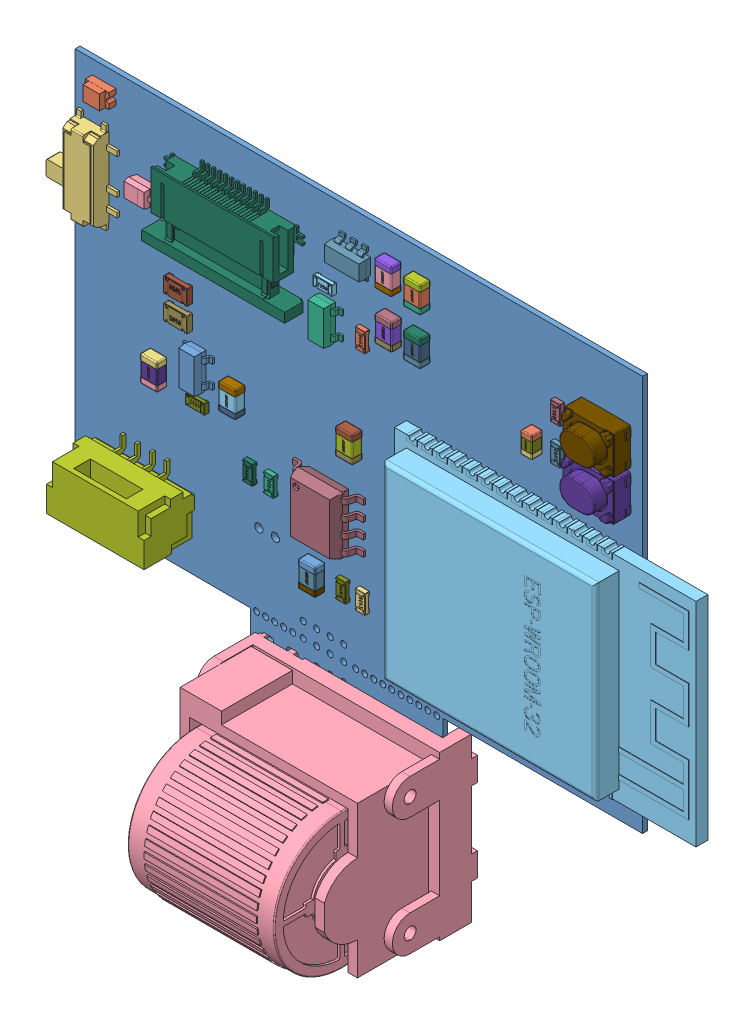
SolidWorks assembly PCB_deskclok_ext_2021-02-23, configuration 默认. Lengths in mm.
Overall size (54.77 48.92 16.75).
124 component instances, 79 part files, 0 mates.
Components (placement in the parent):
- PCB_deskclok_ext_2021-02-23(2)^PCB_deskclok_ext_2021-02-23-1: PCB_deskclok_ext_2021-02-23(2)^PCB_deskclok_ext_2021-02-23 [默认] at origin size (54.77 48.92 16.75) (virtual)
  - Board^PCB_deskclok_ext_2021-02-23(2)_PCB_deskclok_ext_2021-02-23-1: Board^PCB_deskclok_ext_2021-02-23(2)_PCB_deskclok_ext_2021-02-23 [默认] at origin size (48 48.92 0.41) (virtual)
    - Open CASCADE STEP translator 6.8 2.1.1^Board_PCB_deskclok_ext_2021-02-23(2)_PCB_deskclok_ext_2021-02-23-1: Open CASCADE STEP translator 6.8 2.1.1^Board_PCB_deskclok_ext_2021-02-23(2)_PCB_deskclok_ext_2021-02-23 [默认] at (0 0 -0.4115) size (48 48.92 0.41) (virtual)
      - Open CASCADE STEP translator 6.8 2.1.1.1^Open CASCADE STEP translator 6.8 2.1.1_Board_PCB_deskclok_ext_2021-02-23(2)_PCB_deskclok_ext_2021-02-23-1: Open CASCADE STEP translator 6.8 2.1.1.1^Open CASCADE STEP translator 6.8 2.1.1_Board_PCB_deskclok_ext_2021-02-23(2)_PCB_deskclok_ext_2021-02-23 [默认] at origin size (48 48.92 0.41) (virtual)
  - LED6^PCB_deskclok_ext_2021-02-23(2)_PCB_deskclok_ext_2021-02-23-1: LED6^PCB_deskclok_ext_2021-02-23(2)_PCB_deskclok_ext_2021-02-23 [默认] at origin size (2.13 1.25 1.24) (virtual)
    - everlight-17-21-0805LED-GREEN^LED6_PCB_deskclok_ext_2021-02-23(2)_PCB_deskclok_ext_2021-02-23-1: everlight-17-21-0805LED-GREEN^LED6_PCB_deskclok_ext_2021-02-23(2)_PCB_deskclok_ext_2021-02-23 [默认] at (47.3416 90.4196 0.3048) x (1 0 0) z (0 -1 0) size (2.13 1.24 1.25) (virtual)
  - R9^PCB_deskclok_ext_2021-02-23(2)_PCB_deskclok_ext_2021-02-23-1: R9^PCB_deskclok_ext_2021-02-23(2)_PCB_deskclok_ext_2021-02-23 [默认] at origin size (0.8 1.6 0.42) (virtual)
    - User_Library-Res-0603^R9_PCB_deskclok_ext_2021-02-23(2)_PCB_deskclok_ext_2021-02-23-1: User_Library-Res-0603^R9_PCB_deskclok_ext_2021-02-23(2)_PCB_deskclok_ext_2021-02-23 [默认] at (69.3811 64.135 0) x (0 -1 0) z (-1 0 0) size (1.6 0.42 0.8) (virtual)
  - C6^PCB_deskclok_ext_2021-02-23(2)_PCB_deskclok_ext_2021-02-23-1: C6^PCB_deskclok_ext_2021-02-23(2)_PCB_deskclok_ext_2021-02-23 [默认] at origin size (1.45 2.2 0.88) (virtual)
    - c0805c101k5gactu^C6_PCB_deskclok_ext_2021-02-23(2)_PCB_deskclok_ext_2021-02-23-1: c0805c101k5gactu^C6_PCB_deskclok_ext_2021-02-23(2)_PCB_deskclok_ext_2021-02-23 [默认] at (28.223 186.145 -10.6426) x (0 1 0) z (1 0 0) size (2.2 0.88 1.45) (virtual)
      - Open CASCADE STEP translator 6.8 2.4.1.1^c0805c101k5gactu_C6_PCB_deskclok_ext_2021-02-23(2)_PCB_deskclok_ext_2021-02-23-1: Open CASCADE STEP translator 6.8 2.4.1.1^c0805c101k5gactu_C6_PCB_deskclok_ext_2021-02-23(2)_PCB_deskclok_ext_2021-02-23 [默认] at origin size (2 0.86 1.43) (virtual)
      - Open CASCADE STEP translator 6.8 2.4.1.2^c0805c101k5gactu_C6_PCB_deskclok_ext_2021-02-23(2)_PCB_deskclok_ext_2021-02-23-1: Open CASCADE STEP translator 6.8 2.4.1.2^c0805c101k5gactu_C6_PCB_deskclok_ext_2021-02-23(2)_PCB_deskclok_ext_2021-02-23 [默认] at origin size (0.34 0 0.18) (virtual)
      - Open CASCADE STEP translator 6.8 2.4.1.3^c0805c101k5gactu_C6_PCB_deskclok_ext_2021-02-23(2)_PCB_deskclok_ext_2021-02-23-1: Open CASCADE STEP translator 6.8 2.4.1.3^c0805c101k5gactu_C6_PCB_deskclok_ext_2021-02-23(2)_PCB_deskclok_ext_2021-02-23 [默认] at origin size (0.41 0 0.18) (virtual)
      - Open CASCADE STEP translator 6.8 2.4.1.4^c0805c101k5gactu_C6_PCB_deskclok_ext_2021-02-23(2)_PCB_deskclok_ext_2021-02-23-1: Open CASCADE STEP translator 6.8 2.4.1.4^c0805c101k5gactu_C6_PCB_deskclok_ext_2021-02-23(2)_PCB_deskclok_ext_2021-02-23 [默认] at origin size (0.21 0 0.18) (virtual)
      - Open CASCADE STEP translator 6.8 2.4.1.5^c0805c101k5gactu_C6_PCB_deskclok_ext_2021-02-23(2)_PCB_deskclok_ext_2021-02-23-1: Open CASCADE STEP translator 6.8 2.4.1.5^c0805c101k5gactu_C6_PCB_deskclok_ext_2021-02-23(2)_PCB_deskclok_ext_2021-02-23 [默认] at origin size (0.5 0.88 1.45) (virtual)
      - Open CASCADE STEP translator 6.8 2.4.1.6^c0805c101k5gactu_C6_PCB_deskclok_ext_2021-02-23(2)_PCB_deskclok_ext_2021-02-23-1: Open CASCADE STEP translator 6.8 2.4.1.6^c0805c101k5gactu_C6_PCB_deskclok_ext_2021-02-23(2)_PCB_deskclok_ext_2021-02-23 [默认] at origin size (0.5 0.88 1.45) (virtual)
  - C9^PCB_deskclok_ext_2021-02-23(2)_PCB_deskclok_ext_2021-02-23-1: C9^PCB_deskclok_ext_2021-02-23(2)_PCB_deskclok_ext_2021-02-23 [默认] at origin size (1.45 2.2 0.88) (virtual)
    - c0805c101k5gactu^C9_PCB_deskclok_ext_2021-02-23(2)_PCB_deskclok_ext_2021-02-23-1: c0805c101k5gactu^C9_PCB_deskclok_ext_2021-02-23(2)_PCB_deskclok_ext_2021-02-23 [默认] at (117.778 -11.52 -10.6426) x (0 -1 0) z (-1 0 0) size (2.2 0.88 1.45) (virtual)
      - Open CASCADE STEP translator 6.8 2.4.1.1^c0805c101k5gactu_C9_PCB_deskclok_ext_2021-02-23(2)_PCB_deskclok_ext_2021-02-23-1: Open CASCADE STEP translator 6.8 2.4.1.1^c0805c101k5gactu_C9_PCB_deskclok_ext_2021-02-23(2)_PCB_deskclok_ext_2021-02-23 [默认] at origin size (2 0.86 1.43) (virtual)
      - Open CASCADE STEP translator 6.8 2.4.1.2^c0805c101k5gactu_C9_PCB_deskclok_ext_2021-02-23(2)_PCB_deskclok_ext_2021-02-23-1: Open CASCADE STEP translator 6.8 2.4.1.2^c0805c101k5gactu_C9_PCB_deskclok_ext_2021-02-23(2)_PCB_deskclok_ext_2021-02-23 [默认] at origin size (0.34 0 0.18) (virtual)
      - Open CASCADE STEP translator 6.8 2.4.1.3^c0805c101k5gactu_C9_PCB_deskclok_ext_2021-02-23(2)_PCB_deskclok_ext_2021-02-23-1: Open CASCADE STEP translator 6.8 2.4.1.3^c0805c101k5gactu_C9_PCB_deskclok_ext_2021-02-23(2)_PCB_deskclok_ext_2021-02-23 [默认] at origin size (0.41 0 0.18) (virtual)
      - Open CASCADE STEP translator 6.8 2.4.1.4^c0805c101k5gactu_C9_PCB_deskclok_ext_2021-02-23(2)_PCB_deskclok_ext_2021-02-23-1: Open CASCADE STEP translator 6.8 2.4.1.4^c0805c101k5gactu_C9_PCB_deskclok_ext_2021-02-23(2)_PCB_deskclok_ext_2021-02-23 [默认] at origin size (0.21 0 0.18) (virtual)
      - Open CASCADE STEP translator 6.8 2.4.1.5^c0805c101k5gactu_C9_PCB_deskclok_ext_2021-02-23(2)_PCB_deskclok_ext_2021-02-23-1: Open CASCADE STEP translator 6.8 2.4.1.5^c0805c101k5gactu_C9_PCB_deskclok_ext_2021-02-23(2)_PCB_deskclok_ext_2021-02-23 [默认] at origin size (0.5 0.88 1.45) (virtual)
      - Open CASCADE STEP translator 6.8 2.4.1.6^c0805c101k5gactu_C9_PCB_deskclok_ext_2021-02-23(2)_PCB_deskclok_ext_2021-02-23-1: Open CASCADE STEP translator 6.8 2.4.1.6^c0805c101k5gactu_C9_PCB_deskclok_ext_2021-02-23(2)_PCB_deskclok_ext_2021-02-23 [默认] at origin size (0.5 0.88 1.45) (virtual)
  - R1^PCB_deskclok_ext_2021-02-23(2)_PCB_deskclok_ext_2021-02-23-1: R1^PCB_deskclok_ext_2021-02-23(2)_PCB_deskclok_ext_2021-02-23 [默认] at origin size (1.6 0.8 0.42) (virtual)
    - User_Library-Res-0603^R1_PCB_deskclok_ext_2021-02-23(2)_PCB_deskclok_ext_2021-02-23-1: User_Library-Res-0603^R1_PCB_deskclok_ext_2021-02-23(2)_PCB_deskclok_ext_2021-02-23 [默认] at (55.411 71.6281 0) x (1 0 0) z (0 -1 0) size (1.6 0.42 0.8) (virtual)
  - C1^PCB_deskclok_ext_2021-02-23(2)_PCB_deskclok_ext_2021-02-23-1: C1^PCB_deskclok_ext_2021-02-23(2)_PCB_deskclok_ext_2021-02-23 [默认] at origin size (1.45 2.2 0.88) (virtual)
    - c0805c101k5gactu^C1_PCB_deskclok_ext_2021-02-23(2)_PCB_deskclok_ext_2021-02-23-1: c0805c101k5gactu^C1_PCB_deskclok_ext_2021-02-23(2)_PCB_deskclok_ext_2021-02-23 [默认] at (8.411 169.254 -10.6426) x (0 1 0) z (1 0 0) size (2.2 0.88 1.45) (virtual)
      - Open CASCADE STEP translator 6.8 2.4.1.1^c0805c101k5gactu_C1_PCB_deskclok_ext_2021-02-23(2)_PCB_deskclok_ext_2021-02-23-1: Open CASCADE STEP translator 6.8 2.4.1.1^c0805c101k5gactu_C1_PCB_deskclok_ext_2021-02-23(2)_PCB_deskclok_ext_2021-02-23 [默认] at origin size (2 0.86 1.43) (virtual)
      - Open CASCADE STEP translator 6.8 2.4.1.2^c0805c101k5gactu_C1_PCB_deskclok_ext_2021-02-23(2)_PCB_deskclok_ext_2021-02-23-1: Open CASCADE STEP translator 6.8 2.4.1.2^c0805c101k5gactu_C1_PCB_deskclok_ext_2021-02-23(2)_PCB_deskclok_ext_2021-02-23 [默认] at origin size (0.34 0 0.18) (virtual)
      - Open CASCADE STEP translator 6.8 2.4.1.3^c0805c101k5gactu_C1_PCB_deskclok_ext_2021-02-23(2)_PCB_deskclok_ext_2021-02-23-1: Open CASCADE STEP translator 6.8 2.4.1.3^c0805c101k5gactu_C1_PCB_deskclok_ext_2021-02-23(2)_PCB_deskclok_ext_2021-02-23 [默认] at origin size (0.41 0 0.18) (virtual)
      - Open CASCADE STEP translator 6.8 2.4.1.4^c0805c101k5gactu_C1_PCB_deskclok_ext_2021-02-23(2)_PCB_deskclok_ext_2021-02-23-1: Open CASCADE STEP translator 6.8 2.4.1.4^c0805c101k5gactu_C1_PCB_deskclok_ext_2021-02-23(2)_PCB_deskclok_ext_2021-02-23 [默认] at origin size (0.21 0 0.18) (virtual)
      - Open CASCADE STEP translator 6.8 2.4.1.5^c0805c101k5gactu_C1_PCB_deskclok_ext_2021-02-23(2)_PCB_deskclok_ext_2021-02-23-1: Open CASCADE STEP translator 6.8 2.4.1.5^c0805c101k5gactu_C1_PCB_deskclok_ext_2021-02-23(2)_PCB_deskclok_ext_2021-02-23 [默认] at origin size (0.5 0.88 1.45) (virtual)
      - Open CASCADE STEP translator 6.8 2.4.1.6^c0805c101k5gactu_C1_PCB_deskclok_ext_2021-02-23(2)_PCB_deskclok_ext_2021-02-23-1: Open CASCADE STEP translator 6.8 2.4.1.6^c0805c101k5gactu_C1_PCB_deskclok_ext_2021-02-23(2)_PCB_deskclok_ext_2021-02-23 [默认] at origin size (0.5 0.88 1.45) (virtual)
  - C2^PCB_deskclok_ext_2021-02-23(2)_PCB_deskclok_ext_2021-02-23-1: C2^PCB_deskclok_ext_2021-02-23(2)_PCB_deskclok_ext_2021-02-23 [默认] at origin size (1.45 2.2 0.88) (virtual)
    - c0805c101k5gactu^C2_PCB_deskclok_ext_2021-02-23(2)_PCB_deskclok_ext_2021-02-23-1: c0805c101k5gactu^C2_PCB_deskclok_ext_2021-02-23(2)_PCB_deskclok_ext_2021-02-23 [默认] at (15.015 170.524 -10.6426) x (0 1 0) z (1 0 0) size (2.2 0.88 1.45) (virtual)
      - Open CASCADE STEP translator 6.8 2.4.1.1^c0805c101k5gactu_C2_PCB_deskclok_ext_2021-02-23(2)_PCB_deskclok_ext_2021-02-23-1: Open CASCADE STEP translator 6.8 2.4.1.1^c0805c101k5gactu_C2_PCB_deskclok_ext_2021-02-23(2)_PCB_deskclok_ext_2021-02-23 [默认] at origin size (2 0.86 1.43) (virtual)
      - Open CASCADE STEP translator 6.8 2.4.1.2^c0805c101k5gactu_C2_PCB_deskclok_ext_2021-02-23(2)_PCB_deskclok_ext_2021-02-23-1: Open CASCADE STEP translator 6.8 2.4.1.2^c0805c101k5gactu_C2_PCB_deskclok_ext_2021-02-23(2)_PCB_deskclok_ext_2021-02-23 [默认] at origin size (0.34 0 0.18) (virtual)
      - Open CASCADE STEP translator 6.8 2.4.1.3^c0805c101k5gactu_C2_PCB_deskclok_ext_2021-02-23(2)_PCB_deskclok_ext_2021-02-23-1: Open CASCADE STEP translator 6.8 2.4.1.3^c0805c101k5gactu_C2_PCB_deskclok_ext_2021-02-23(2)_PCB_deskclok_ext_2021-02-23 [默认] at origin size (0.41 0 0.18) (virtual)
      - Open CASCADE STEP translator 6.8 2.4.1.4^c0805c101k5gactu_C2_PCB_deskclok_ext_2021-02-23(2)_PCB_deskclok_ext_2021-02-23-1: Open CASCADE STEP translator 6.8 2.4.1.4^c0805c101k5gactu_C2_PCB_deskclok_ext_2021-02-23(2)_PCB_deskclok_ext_2021-02-23 [默认] at origin size (0.21 0 0.18) (virtual)
      - Open CASCADE STEP translator 6.8 2.4.1.5^c0805c101k5gactu_C2_PCB_deskclok_ext_2021-02-23(2)_PCB_deskclok_ext_2021-02-23-1: Open CASCADE STEP translator 6.8 2.4.1.5^c0805c101k5gactu_C2_PCB_deskclok_ext_2021-02-23(2)_PCB_deskclok_ext_2021-02-23 [默认] at origin size (0.5 0.88 1.45) (virtual)
      - Open CASCADE STEP translator 6.8 2.4.1.6^c0805c101k5gactu_C2_PCB_deskclok_ext_2021-02-23(2)_PCB_deskclok_ext_2021-02-23-1: Open CASCADE STEP translator 6.8 2.4.1.6^c0805c101k5gactu_C2_PCB_deskclok_ext_2021-02-23(2)_PCB_deskclok_ext_2021-02-23 [默认] at origin size (0.5 0.88 1.45) (virtual)
  - R13^PCB_deskclok_ext_2021-02-23(2)_PCB_deskclok_ext_2021-02-23-1: R13^PCB_deskclok_ext_2021-02-23(2)_PCB_deskclok_ext_2021-02-23 [默认] at origin size (2 1.25 0.53) (virtual)
    - User_Library-Res-0805^R13_PCB_deskclok_ext_2021-02-23(2)_PCB_deskclok_ext_2021-02-23-1: User_Library-Res-0805^R13_PCB_deskclok_ext_2021-02-23(2)_PCB_deskclok_ext_2021-02-23 [默认] at (54.1409 79.4919 0.3048) x (1 0 0) z (0 -1 0) size (2 0.53 1.25) (virtual)
  - R14^PCB_deskclok_ext_2021-02-23(2)_PCB_deskclok_ext_2021-02-23-1: R14^PCB_deskclok_ext_2021-02-23(2)_PCB_deskclok_ext_2021-02-23 [默认] at origin size (2 1.25 0.53) (virtual)
    - User_Library-Res-0805^R14_PCB_deskclok_ext_2021-02-23(2)_PCB_deskclok_ext_2021-02-23-1: User_Library-Res-0805^R14_PCB_deskclok_ext_2021-02-23(2)_PCB_deskclok_ext_2021-02-23 [默认] at (54.141 77.4801 0.3048) x (-1 0 0) z (0 1 0) size (2 0.53 1.25) (virtual)
  - U3^PCB_deskclok_ext_2021-02-23(2)_PCB_deskclok_ext_2021-02-23-1: U3^PCB_deskclok_ext_2021-02-23(2)_PCB_deskclok_ext_2021-02-23 [默认] at origin size (6 4.9 1.7) (virtual)
    - User_Library-so8-3^U3_PCB_deskclok_ext_2021-02-23(2)_PCB_deskclok_ext_2021-02-23-1: User_Library-so8-3^U3_PCB_deskclok_ext_2021-02-23(2)_PCB_deskclok_ext_2021-02-23 [默认] at (66.4601 69.469 0) x (1 0 0) z (0 0 1) size (6 4.9 1.7) (virtual)
  - U9^PCB_deskclok_ext_2021-02-23(2)_PCB_deskclok_ext_2021-02-23-1: U9^PCB_deskclok_ext_2021-02-23(2)_PCB_deskclok_ext_2021-02-23 [默认] at origin size (3 2.5 1.1) (virtual)
    - CircuitWorks-SOT-23-5^U9_PCB_deskclok_ext_2021-02-23(2)_PCB_deskclok_ext_2021-02-23-1: CircuitWorks-SOT-23-5^U9_PCB_deskclok_ext_2021-02-23(2)_PCB_deskclok_ext_2021-02-23 [默认] at (68.536 88.8961 0.5588) x (-1 0 0) z (0 1 0) size (3 1.1 2.5) (virtual)
  - FPC3^PCB_deskclok_ext_2021-02-23(2)_PCB_deskclok_ext_2021-02-23-1: FPC3^PCB_deskclok_ext_2021-02-23(2)_PCB_deskclok_ext_2021-02-23 [默认] at origin size (12.1 6.6 2) (virtual)
    - 52746-1290_RGB10066329^FPC3_PCB_deskclok_ext_2021-02-23(2)_PCB_deskclok_ext_2021-02-23-1: 52746-1290_RGB10066329^FPC3_PCB_deskclok_ext_2021-02-23(2)_PCB_deskclok_ext_2021-02-23 [默认] at (58.4591 88.7731 0) x (1 0 0) z (0 -1 0) size (12.1 2 6.6) (virtual)
  - C35^PCB_deskclok_ext_2021-02-23(2)_PCB_deskclok_ext_2021-02-23-1: C35^PCB_deskclok_ext_2021-02-23(2)_PCB_deskclok_ext_2021-02-23 [默认] at origin size (0.95 1.77 0.95) (virtual)
    - c0603x104k3ractu^C35_PCB_deskclok_ext_2021-02-23(2)_PCB_deskclok_ext_2021-02-23-1: c0603x104k3ractu^C35_PCB_deskclok_ext_2021-02-23(2)_PCB_deskclok_ext_2021-02-23 [默认] at (40.1705 179.789 -10.6426) x (0 1 0) z (1 0 0) size (1.77 0.95 0.95) (virtual)
      - Open CASCADE STEP translator 6.8 2.14.1.1^c0603x104k3ractu_C35_PCB_deskclok_ext_2021-02-23(2)_PCB_deskclok_ext_2021-02-23-1: Open CASCADE STEP translator 6.8 2.14.1.1^c0603x104k3ractu_C35_PCB_deskclok_ext_2021-02-23(2)_PCB_deskclok_ext_2021-02-23 [默认] at origin size (1.57 0.93 0.93) (virtual)
      - Open CASCADE STEP translator 6.8 2.14.1.2^c0603x104k3ractu_C35_PCB_deskclok_ext_2021-02-23(2)_PCB_deskclok_ext_2021-02-23-1: Open CASCADE STEP translator 6.8 2.14.1.2^c0603x104k3ractu_C35_PCB_deskclok_ext_2021-02-23(2)_PCB_deskclok_ext_2021-02-23 [默认] at origin size (0.24 0 0.13) (virtual)
      - Open CASCADE STEP translator 6.8 2.14.1.3^c0603x104k3ractu_C35_PCB_deskclok_ext_2021-02-23(2)_PCB_deskclok_ext_2021-02-23-1: Open CASCADE STEP translator 6.8 2.14.1.3^c0603x104k3ractu_C35_PCB_deskclok_ext_2021-02-23(2)_PCB_deskclok_ext_2021-02-23 [默认] at origin size (0.29 0 0.13) (virtual)
      - Open CASCADE STEP translator 6.8 2.14.1.4^c0603x104k3ractu_C35_PCB_deskclok_ext_2021-02-23(2)_PCB_deskclok_ext_2021-02-23-1: Open CASCADE STEP translator 6.8 2.14.1.4^c0603x104k3ractu_C35_PCB_deskclok_ext_2021-02-23(2)_PCB_deskclok_ext_2021-02-23 [默认] at origin size (0.15 0 0.13) (virtual)
      - Open CASCADE STEP translator 6.8 2.14.1.5^c0603x104k3ractu_C35_PCB_deskclok_ext_2021-02-23(2)_PCB_deskclok_ext_2021-02-23-1: Open CASCADE STEP translator 6.8 2.14.1.5^c0603x104k3ractu_C35_PCB_deskclok_ext_2021-02-23(2)_PCB_deskclok_ext_2021-02-23 [默认] at origin size (0.45 0.95 0.95) (virtual)
      - Open CASCADE STEP translator 6.8 2.14.1.6^c0603x104k3ractu_C35_PCB_deskclok_ext_2021-02-23(2)_PCB_deskclok_ext_2021-02-23-1: Open CASCADE STEP translator 6.8 2.14.1.6^c0603x104k3ractu_C35_PCB_deskclok_ext_2021-02-23(2)_PCB_deskclok_ext_2021-02-23 [默认] at origin size (0.45 0.95 0.95) (virtual)
  - D1^PCB_deskclok_ext_2021-02-23(2)_PCB_deskclok_ext_2021-02-23-1: D1^PCB_deskclok_ext_2021-02-23(2)_PCB_deskclok_ext_2021-02-23 [默认] at origin size (2.6 1.35 1.1) (virtual)
    - User_Library-SOD323-1^D1_PCB_deskclok_ext_2021-02-23(2)_PCB_deskclok_ext_2021-02-23-1: User_Library-SOD323-1^D1_PCB_deskclok_ext_2021-02-23(2)_PCB_deskclok_ext_2021-02-23 [默认] at (50.9659 85.0899 0) x (-1 0 0) z (0 0 1) size (2.6 1.35 1.1) (virtual)
  - R4^PCB_deskclok_ext_2021-02-23(2)_PCB_deskclok_ext_2021-02-23-1: R4^PCB_deskclok_ext_2021-02-23(2)_PCB_deskclok_ext_2021-02-23 [默认] at origin size (1.6 0.8 0.42) (virtual)
    - User_Library-Res-0603^R4_PCB_deskclok_ext_2021-02-23(2)_PCB_deskclok_ext_2021-02-23-1: User_Library-Res-0603^R4_PCB_deskclok_ext_2021-02-23(2)_PCB_deskclok_ext_2021-02-23 [默认] at (66.2059 85.7249 0) x (-1 0 0) z (0 1 0) size (1.6 0.42 0.8) (virtual)
  - R8^PCB_deskclok_ext_2021-02-23(2)_PCB_deskclok_ext_2021-02-23-1: R8^PCB_deskclok_ext_2021-02-23(2)_PCB_deskclok_ext_2021-02-23 [默认] at origin size (0.8 1.6 0.42) (virtual)
    - User_Library-Res-0603^R8_PCB_deskclok_ext_2021-02-23(2)_PCB_deskclok_ext_2021-02-23-1: User_Library-Res-0603^R8_PCB_deskclok_ext_2021-02-23(2)_PCB_deskclok_ext_2021-02-23 [默认] at (61.6341 68.834 0) x (0 -1 0) z (-1 0 0) size (1.6 0.42 0.8) (virtual)
  - C4^PCB_deskclok_ext_2021-02-23(2)_PCB_deskclok_ext_2021-02-23-1: C4^PCB_deskclok_ext_2021-02-23(2)_PCB_deskclok_ext_2021-02-23 [默认] at origin size (1.45 2.2 0.88) (virtual)
    - c0805c101k5gactu^C4_PCB_deskclok_ext_2021-02-23(2)_PCB_deskclok_ext_2021-02-23-1: c0805c101k5gactu^C4_PCB_deskclok_ext_2021-02-23(2)_PCB_deskclok_ext_2021-02-23 [默认] at (24.921 172.175 -10.6426) x (0 1 0) z (1 0 0) size (2.2 0.88 1.45) (virtual)
      - Open CASCADE STEP translator 6.8 2.4.1.1^c0805c101k5gactu_C4_PCB_deskclok_ext_2021-02-23(2)_PCB_deskclok_ext_2021-02-23-1: Open CASCADE STEP translator 6.8 2.4.1.1^c0805c101k5gactu_C4_PCB_deskclok_ext_2021-02-23(2)_PCB_deskclok_ext_2021-02-23 [默认] at origin size (2 0.86 1.43) (virtual)
      - Open CASCADE STEP translator 6.8 2.4.1.2^c0805c101k5gactu_C4_PCB_deskclok_ext_2021-02-23(2)_PCB_deskclok_ext_2021-02-23-1: Open CASCADE STEP translator 6.8 2.4.1.2^c0805c101k5gactu_C4_PCB_deskclok_ext_2021-02-23(2)_PCB_deskclok_ext_2021-02-23 [默认] at origin size (0.34 0 0.18) (virtual)
      - Open CASCADE STEP translator 6.8 2.4.1.3^c0805c101k5gactu_C4_PCB_deskclok_ext_2021-02-23(2)_PCB_deskclok_ext_2021-02-23-1: Open CASCADE STEP translator 6.8 2.4.1.3^c0805c101k5gactu_C4_PCB_deskclok_ext_2021-02-23(2)_PCB_deskclok_ext_2021-02-23 [默认] at origin size (0.41 0 0.18) (virtual)
      - Open CASCADE STEP translator 6.8 2.4.1.4^c0805c101k5gactu_C4_PCB_deskclok_ext_2021-02-23(2)_PCB_deskclok_ext_2021-02-23-1: Open CASCADE STEP translator 6.8 2.4.1.4^c0805c101k5gactu_C4_PCB_deskclok_ext_2021-02-23(2)_PCB_deskclok_ext_2021-02-23 [默认] at origin size (0.21 0 0.18) (virtual)
      - Open CASCADE STEP translator 6.8 2.4.1.5^c0805c101k5gactu_C4_PCB_deskclok_ext_2021-02-23(2)_PCB_deskclok_ext_2021-02-23-1: Open CASCADE STEP translator 6.8 2.4.1.5^c0805c101k5gactu_C4_PCB_deskclok_ext_2021-02-23(2)_PCB_deskclok_ext_2021-02-23 [默认] at origin size (0.5 0.88 1.45) (virtual)
      - Open CASCADE STEP translator 6.8 2.4.1.6^c0805c101k5gactu_C4_PCB_deskclok_ext_2021-02-23(2)_PCB_deskclok_ext_2021-02-23-1: Open CASCADE STEP translator 6.8 2.4.1.6^c0805c101k5gactu_C4_PCB_deskclok_ext_2021-02-23(2)_PCB_deskclok_ext_2021-02-23 [默认] at origin size (0.5 0.88 1.45) (virtual)
  - R7^PCB_deskclok_ext_2021-02-23(2)_PCB_deskclok_ext_2021-02-23-1: R7^PCB_deskclok_ext_2021-02-23(2)_PCB_deskclok_ext_2021-02-23 [默认] at origin size (0.8 1.6 0.42) (virtual)
    - User_Library-Res-0603^R7_PCB_deskclok_ext_2021-02-23(2)_PCB_deskclok_ext_2021-02-23-1: User_Library-Res-0603^R7_PCB_deskclok_ext_2021-02-23(2)_PCB_deskclok_ext_2021-02-23 [默认] at (85.8909 86.233 0) x (0 1 0) z (1 0 0) size (1.6 0.42 0.8) (virtual)
  - R6^PCB_deskclok_ext_2021-02-23(2)_PCB_deskclok_ext_2021-02-23-1: R6^PCB_deskclok_ext_2021-02-23(2)_PCB_deskclok_ext_2021-02-23 [默认] at origin size (0.8 1.6 0.42) (virtual)
    - User_Library-Res-0603^R6_PCB_deskclok_ext_2021-02-23(2)_PCB_deskclok_ext_2021-02-23-1: User_Library-Res-0603^R6_PCB_deskclok_ext_2021-02-23(2)_PCB_deskclok_ext_2021-02-23 [默认] at (85.8911 83.185 0) x (0 -1 0) z (-1 0 0) size (1.6 0.42 0.8) (virtual)
  - R3^PCB_deskclok_ext_2021-02-23(2)_PCB_deskclok_ext_2021-02-23-1: R3^PCB_deskclok_ext_2021-02-23(2)_PCB_deskclok_ext_2021-02-23 [默认] at origin size (0.8 1.6 0.42) (virtual)
    - User_Library-Res-0603^R3_PCB_deskclok_ext_2021-02-23(2)_PCB_deskclok_ext_2021-02-23-1: User_Library-Res-0603^R3_PCB_deskclok_ext_2021-02-23(2)_PCB_deskclok_ext_2021-02-23 [默认] at (59.8559 68.834 0) x (0 1 0) z (1 0 0) size (1.6 0.42 0.8) (virtual)
  - R2^PCB_deskclok_ext_2021-02-23(2)_PCB_deskclok_ext_2021-02-23-1: R2^PCB_deskclok_ext_2021-02-23(2)_PCB_deskclok_ext_2021-02-23 [默认] at origin size (0.8 1.6 0.42) (virtual)
    - User_Library-Res-0603^R2_PCB_deskclok_ext_2021-02-23(2)_PCB_deskclok_ext_2021-02-23-1: User_Library-Res-0603^R2_PCB_deskclok_ext_2021-02-23(2)_PCB_deskclok_ext_2021-02-23 [默认] at (67.7301 64.135 0) x (0 -1 0) z (-1 0 0) size (1.6 0.42 0.8) (virtual)
  - SW1^PCB_deskclok_ext_2021-02-23(2)_PCB_deskclok_ext_2021-02-23-1: SW1^PCB_deskclok_ext_2021-02-23(2)_PCB_deskclok_ext_2021-02-23 [默认] at origin size (4.6 3.2 2.5) (virtual)
    - skrpace010_RGB10066329^SW1_PCB_deskclok_ext_2021-02-23(2)_PCB_deskclok_ext_2021-02-23-1: skrpace010_RGB10066329^SW1_PCB_deskclok_ext_2021-02-23(2)_PCB_deskclok_ext_2021-02-23 [默认] at (89.8279 83.185 0) x (-1 0 0) z (0 1 0) size (4.6 2.5 3.2) (virtual)
  - SW2^PCB_deskclok_ext_2021-02-23(2)_PCB_deskclok_ext_2021-02-23-1: SW2^PCB_deskclok_ext_2021-02-23(2)_PCB_deskclok_ext_2021-02-23 [默认] at origin size (4.6 3.2 2.5) (virtual)
    - skrpace010_RGB10066329^SW2_PCB_deskclok_ext_2021-02-23(2)_PCB_deskclok_ext_2021-02-23-1: skrpace010_RGB10066329^SW2_PCB_deskclok_ext_2021-02-23(2)_PCB_deskclok_ext_2021-02-23 [默认] at (89.8281 86.614 0) x (1 0 0) z (0 -1 0) size (4.6 2.5 3.2) (virtual)
  - U1^PCB_deskclok_ext_2021-02-23(2)_PCB_deskclok_ext_2021-02-23-1: U1^PCB_deskclok_ext_2021-02-23(2)_PCB_deskclok_ext_2021-02-23 [默认] at origin size (2.5 3 1.1) (virtual)
    - CircuitWorks-SOT-23-5^U1_PCB_deskclok_ext_2021-02-23(2)_PCB_deskclok_ext_2021-02-23-1: CircuitWorks-SOT-23-5^U1_PCB_deskclok_ext_2021-02-23(2)_PCB_deskclok_ext_2021-02-23 [默认] at (55.4148 74.339 0.5588) x (0 -1 0) z (-1 0 0) size (3 1.1 2.5) (virtual)
  - C7^PCB_deskclok_ext_2021-02-23(2)_PCB_deskclok_ext_2021-02-23-1: C7^PCB_deskclok_ext_2021-02-23(2)_PCB_deskclok_ext_2021-02-23 [默认] at origin size (1.45 2.2 0.88) (virtual)
    - c0805c101k5gactu^C7_PCB_deskclok_ext_2021-02-23(2)_PCB_deskclok_ext_2021-02-23-1: c0805c101k5gactu^C7_PCB_deskclok_ext_2021-02-23(2)_PCB_deskclok_ext_2021-02-23 [默认] at (117.778 -7.583 -10.6426) x (0 -1 0) z (-1 0 0) size (2.2 0.88 1.45) (virtual)
      - Open CASCADE STEP translator 6.8 2.4.1.1^c0805c101k5gactu_C7_PCB_deskclok_ext_2021-02-23(2)_PCB_deskclok_ext_2021-02-23-1: Open CASCADE STEP translator 6.8 2.4.1.1^c0805c101k5gactu_C7_PCB_deskclok_ext_2021-02-23(2)_PCB_deskclok_ext_2021-02-23 [默认] at origin size (2 0.86 1.43) (virtual)
      - Open CASCADE STEP translator 6.8 2.4.1.2^c0805c101k5gactu_C7_PCB_deskclok_ext_2021-02-23(2)_PCB_deskclok_ext_2021-02-23-1: Open CASCADE STEP translator 6.8 2.4.1.2^c0805c101k5gactu_C7_PCB_deskclok_ext_2021-02-23(2)_PCB_deskclok_ext_2021-02-23 [默认] at origin size (0.34 0 0.18) (virtual)
      - Open CASCADE STEP translator 6.8 2.4.1.3^c0805c101k5gactu_C7_PCB_deskclok_ext_2021-02-23(2)_PCB_deskclok_ext_2021-02-23-1: Open CASCADE STEP translator 6.8 2.4.1.3^c0805c101k5gactu_C7_PCB_deskclok_ext_2021-02-23(2)_PCB_deskclok_ext_2021-02-23 [默认] at origin size (0.41 0 0.18) (virtual)
      - Open CASCADE STEP translator 6.8 2.4.1.4^c0805c101k5gactu_C7_PCB_deskclok_ext_2021-02-23(2)_PCB_deskclok_ext_2021-02-23-1: Open CASCADE STEP translator 6.8 2.4.1.4^c0805c101k5gactu_C7_PCB_deskclok_ext_2021-02-23(2)_PCB_deskclok_ext_2021-02-23 [默认] at origin size (0.21 0 0.18) (virtual)
      - Open CASCADE STEP translator 6.8 2.4.1.5^c0805c101k5gactu_C7_PCB_deskclok_ext_2021-02-23(2)_PCB_deskclok_ext_2021-02-23-1: Open CASCADE STEP translator 6.8 2.4.1.5^c0805c101k5gactu_C7_PCB_deskclok_ext_2021-02-23(2)_PCB_deskclok_ext_2021-02-23 [默认] at origin size (0.5 0.88 1.45) (virtual)
      - Open CASCADE STEP translator 6.8 2.4.1.6^c0805c101k5gactu_C7_PCB_deskclok_ext_2021-02-23(2)_PCB_deskclok_ext_2021-02-23-1: Open CASCADE STEP translator 6.8 2.4.1.6^c0805c101k5gactu_C7_PCB_deskclok_ext_2021-02-23(2)_PCB_deskclok_ext_2021-02-23 [默认] at origin size (0.5 0.88 1.45) (virtual)
  - C8^PCB_deskclok_ext_2021-02-23(2)_PCB_deskclok_ext_2021-02-23-1: C8^PCB_deskclok_ext_2021-02-23(2)_PCB_deskclok_ext_2021-02-23 [默认] at origin size (1.45 2.2 0.88) (virtual)
    - c0805c101k5gactu^C8_PCB_deskclok_ext_2021-02-23(2)_PCB_deskclok_ext_2021-02-23-1: c0805c101k5gactu^C8_PCB_deskclok_ext_2021-02-23(2)_PCB_deskclok_ext_2021-02-23 [默认] at (115.365 -11.52 -10.6426) x (0 -1 0) z (-1 0 0) size (2.2 0.88 1.45) (virtual)
      - Open CASCADE STEP translator 6.8 2.4.1.1^c0805c101k5gactu_C8_PCB_deskclok_ext_2021-02-23(2)_PCB_deskclok_ext_2021-02-23-1: Open CASCADE STEP translator 6.8 2.4.1.1^c0805c101k5gactu_C8_PCB_deskclok_ext_2021-02-23(2)_PCB_deskclok_ext_2021-02-23 [默认] at origin size (2 0.86 1.43) (virtual)
      - Open CASCADE STEP translator 6.8 2.4.1.2^c0805c101k5gactu_C8_PCB_deskclok_ext_2021-02-23(2)_PCB_deskclok_ext_2021-02-23-1: Open CASCADE STEP translator 6.8 2.4.1.2^c0805c101k5gactu_C8_PCB_deskclok_ext_2021-02-23(2)_PCB_deskclok_ext_2021-02-23 [默认] at origin size (0.34 0 0.18) (virtual)
      - Open CASCADE STEP translator 6.8 2.4.1.3^c0805c101k5gactu_C8_PCB_deskclok_ext_2021-02-23(2)_PCB_deskclok_ext_2021-02-23-1: Open CASCADE STEP translator 6.8 2.4.1.3^c0805c101k5gactu_C8_PCB_deskclok_ext_2021-02-23(2)_PCB_deskclok_ext_2021-02-23 [默认] at origin size (0.41 0 0.18) (virtual)
      - Open CASCADE STEP translator 6.8 2.4.1.4^c0805c101k5gactu_C8_PCB_deskclok_ext_2021-02-23(2)_PCB_deskclok_ext_2021-02-23-1: Open CASCADE STEP translator 6.8 2.4.1.4^c0805c101k5gactu_C8_PCB_deskclok_ext_2021-02-23(2)_PCB_deskclok_ext_2021-02-23 [默认] at origin size (0.21 0 0.18) (virtual)
      - Open CASCADE STEP translator 6.8 2.4.1.5^c0805c101k5gactu_C8_PCB_deskclok_ext_2021-02-23(2)_PCB_deskclok_ext_2021-02-23-1: Open CASCADE STEP translator 6.8 2.4.1.5^c0805c101k5gactu_C8_PCB_deskclok_ext_2021-02-23(2)_PCB_deskclok_ext_2021-02-23 [默认] at origin size (0.5 0.88 1.45) (virtual)
      - Open CASCADE STEP translator 6.8 2.4.1.6^c0805c101k5gactu_C8_PCB_deskclok_ext_2021-02-23(2)_PCB_deskclok_ext_2021-02-23-1: Open CASCADE STEP translator 6.8 2.4.1.6^c0805c101k5gactu_C8_PCB_deskclok_ext_2021-02-23(2)_PCB_deskclok_ext_2021-02-23 [默认] at origin size (0.5 0.88 1.45) (virtual)
  - C3^PCB_deskclok_ext_2021-02-23(2)_PCB_deskclok_ext_2021-02-23-1: C3^PCB_deskclok_ext_2021-02-23(2)_PCB_deskclok_ext_2021-02-23 [默认] at origin size (1.45 2.2 0.88) (virtual)
    - c0805c101k5gactu^C3_PCB_deskclok_ext_2021-02-23(2)_PCB_deskclok_ext_2021-02-23-1: c0805c101k5gactu^C3_PCB_deskclok_ext_2021-02-23(2)_PCB_deskclok_ext_2021-02-23 [默认] at (108.888 -32.729 -10.6426) x (0 -1 0) z (-1 0 0) size (2.2 0.88 1.45) (virtual)
      - Open CASCADE STEP translator 6.8 2.4.1.1^c0805c101k5gactu_C3_PCB_deskclok_ext_2021-02-23(2)_PCB_deskclok_ext_2021-02-23-1: Open CASCADE STEP translator 6.8 2.4.1.1^c0805c101k5gactu_C3_PCB_deskclok_ext_2021-02-23(2)_PCB_deskclok_ext_2021-02-23 [默认] at origin size (2 0.86 1.43) (virtual)
      - Open CASCADE STEP translator 6.8 2.4.1.2^c0805c101k5gactu_C3_PCB_deskclok_ext_2021-02-23(2)_PCB_deskclok_ext_2021-02-23-1: Open CASCADE STEP translator 6.8 2.4.1.2^c0805c101k5gactu_C3_PCB_deskclok_ext_2021-02-23(2)_PCB_deskclok_ext_2021-02-23 [默认] at origin size (0.34 0 0.18) (virtual)
      - Open CASCADE STEP translator 6.8 2.4.1.3^c0805c101k5gactu_C3_PCB_deskclok_ext_2021-02-23(2)_PCB_deskclok_ext_2021-02-23-1: Open CASCADE STEP translator 6.8 2.4.1.3^c0805c101k5gactu_C3_PCB_deskclok_ext_2021-02-23(2)_PCB_deskclok_ext_2021-02-23 [默认] at origin size (0.41 0 0.18) (virtual)
      - Open CASCADE STEP translator 6.8 2.4.1.4^c0805c101k5gactu_C3_PCB_deskclok_ext_2021-02-23(2)_PCB_deskclok_ext_2021-02-23-1: Open CASCADE STEP translator 6.8 2.4.1.4^c0805c101k5gactu_C3_PCB_deskclok_ext_2021-02-23(2)_PCB_deskclok_ext_2021-02-23 [默认] at origin size (0.21 0 0.18) (virtual)
      - Open CASCADE STEP translator 6.8 2.4.1.5^c0805c101k5gactu_C3_PCB_deskclok_ext_2021-02-23(2)_PCB_deskclok_ext_2021-02-23-1: Open CASCADE STEP translator 6.8 2.4.1.5^c0805c101k5gactu_C3_PCB_deskclok_ext_2021-02-23(2)_PCB_deskclok_ext_2021-02-23 [默认] at origin size (0.5 0.88 1.45) (virtual)
      - Open CASCADE STEP translator 6.8 2.4.1.6^c0805c101k5gactu_C3_PCB_deskclok_ext_2021-02-23(2)_PCB_deskclok_ext_2021-02-23-1: Open CASCADE STEP translator 6.8 2.4.1.6^c0805c101k5gactu_C3_PCB_deskclok_ext_2021-02-23(2)_PCB_deskclok_ext_2021-02-23 [默认] at origin size (0.5 0.88 1.45) (virtual)
  - R5^PCB_deskclok_ext_2021-02-23(2)_PCB_deskclok_ext_2021-02-23-1: R5^PCB_deskclok_ext_2021-02-23(2)_PCB_deskclok_ext_2021-02-23 [默认] at origin size (0.8 1.6 0.42) (virtual)
    - User_Library-Res-0603^R5_PCB_deskclok_ext_2021-02-23(2)_PCB_deskclok_ext_2021-02-23-1: User_Library-Res-0603^R5_PCB_deskclok_ext_2021-02-23(2)_PCB_deskclok_ext_2021-02-23 [默认] at (69.3811 83.312 0) x (0 -1 0) z (-1 0 0) size (1.6 0.42 0.8) (virtual)
  - SW3^PCB_deskclok_ext_2021-02-23(2)_PCB_deskclok_ext_2021-02-23-1: SW3^PCB_deskclok_ext_2021-02-23(2)_PCB_deskclok_ext_2021-02-23 [默认] at origin size (5 7.7 1.9) (virtual)
    - User_Library-MSS3_slide_switch_v2^SW3_PCB_deskclok_ext_2021-02-23(2)_PCB_deskclok_ext_2021-02-23-1: User_Library-MSS3_slide_switch_v2^SW3_PCB_deskclok_ext_2021-02-23(2)_PCB_deskclok_ext_2021-02-23 [默认] at (46.3941 83.6929 0) x (0 1 0) z (0 0 1) size (7.7 5 1.9) (virtual)
  - U5^PCB_deskclok_ext_2021-02-23(2)_PCB_deskclok_ext_2021-02-23-1: U5^PCB_deskclok_ext_2021-02-23(2)_PCB_deskclok_ext_2021-02-23 [默认] at origin size (16.6 13.85 16.75) (virtual)
    - Encoder^U5_PCB_deskclok_ext_2021-02-23(2)_PCB_deskclok_ext_2021-02-23-1: Encoder^U5_PCB_deskclok_ext_2021-02-23(2)_PCB_deskclok_ext_2021-02-23 [默认] at (76.9191 43.4839 0) x (0 1 0) z (1 0 0) size (13.85 16.75 16.6) (virtual)
  - U2^PCB_deskclok_ext_2021-02-23(2)_PCB_deskclok_ext_2021-02-23-1: U2^PCB_deskclok_ext_2021-02-23(2)_PCB_deskclok_ext_2021-02-23 [默认] at origin size (25.54 18.07 3.04) (virtual)
    - User_Library-esp-wroom-32^U2_PCB_deskclok_ext_2021-02-23(2)_PCB_deskclok_ext_2021-02-23-1: User_Library-esp-wroom-32^U2_PCB_deskclok_ext_2021-02-23(2)_PCB_deskclok_ext_2021-02-23 [默认] at (72.907 78.995 0) x (0 -1 0) z (-1 0 0) size (18.07 3.04 25.54) (virtual)
  - Q2^PCB_deskclok_ext_2021-02-23(2)_PCB_deskclok_ext_2021-02-23-1: Q2^PCB_deskclok_ext_2021-02-23(2)_PCB_deskclok_ext_2021-02-23 [默认] at origin size (2.5 3 1.1) (virtual)
    - CircuitWorks-SOT-23^Q2_PCB_deskclok_ext_2021-02-23(2)_PCB_deskclok_ext_2021-02-23-1: CircuitWorks-SOT-23^Q2_PCB_deskclok_ext_2021-02-23(2)_PCB_deskclok_ext_2021-02-23 [默认] at (66.3331 83.3121 0.5334) x (0 -1 0) z (-1 0 0) size (3 1.1 2.5) (virtual)
  - CN9^PCB_deskclok_ext_2021-02-23(2)_PCB_deskclok_ext_2021-02-23-1: CN9^PCB_deskclok_ext_2021-02-23(2)_PCB_deskclok_ext_2021-02-23 [默认] at origin size (8.25 4.85 4.35) (virtual)
    - User_Library-SM04B-GHS-TB_RGB8421504^CN9_PCB_deskclok_ext_2021-02-23(2)_PCB_deskclok_ext_2021-02-23-1: User_Library-SM04B-GHS-TB_RGB8421504^CN9_PCB_deskclok_ext_2021-02-23(2)_PCB_deskclok_ext_2021-02-23 [默认] at (55.0909 65.3909 0.127) x (1 0 0) z (0 -1 0) size (8.25 4.35 4.85) (virtual)
